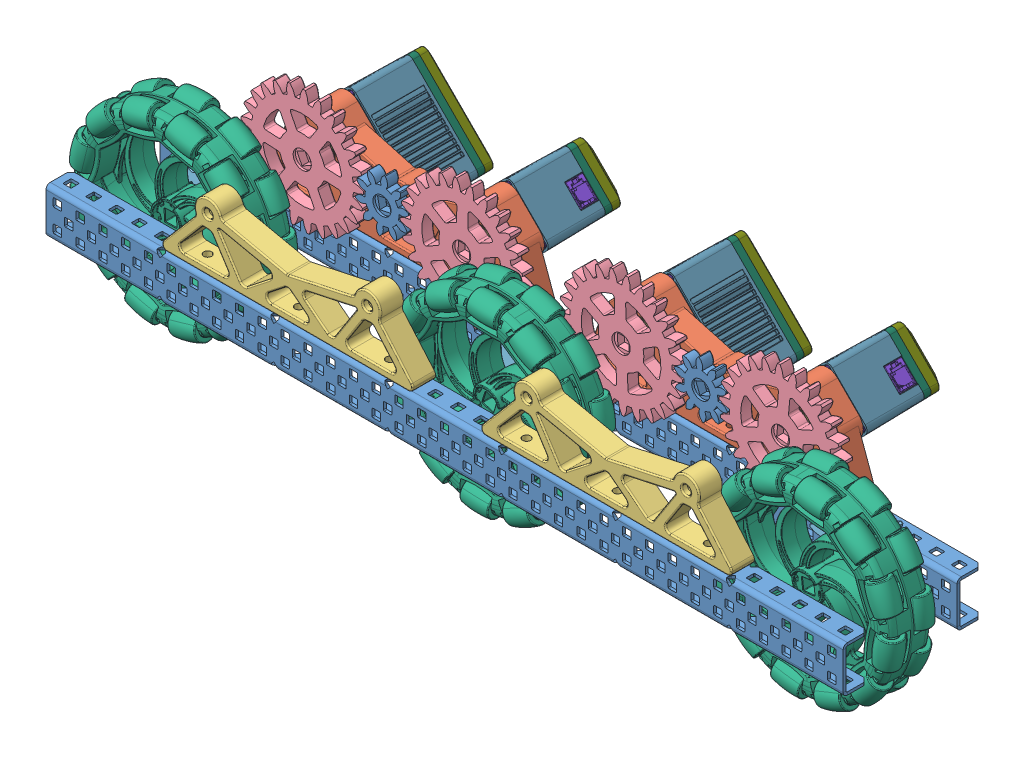
SolidWorks assembly Chassis_Side_assembly, configuration Default. Lengths in mm.
Overall size (477.85 153.68 124.38).
102 component instances, 19 part files, 62 mates.
Components (placement in the parent):
- 1x2x1x35 Aluminum C-Channel (276-2289)-1: 1x2x1x35 Aluminum C-Channel (276-2289) [Default] at (127.7015 217.7804 370.9956) size (444.5 25.41 13.97)
- 1x2x1x35 Aluminum C-Channel (276-2289)-2: 1x2x1x35 Aluminum C-Channel (276-2289) [Default] at (127.7015 217.7804 307.4956) size (444.5 25.41 13.97)
- chassis_inner_bracket-1: chassis_inner_bracket [Default] at (127.7015 224.1304 306.2256) x (-1 0 0) z (0 0 -1) size (150.69 49.95 15.04)
- chassis_inner_bracket-2: chassis_inner_bracket [Default] at (305.5015 224.1304 306.2256) x (-1 0 0) z (0 0 -1) size (150.69 49.95 15.04)
- chassis_outer_bracket-1: chassis_outer_bracket [Default] at (127.7015 224.1304 369.7256) x (-1 0 0) z (0 0 -1) size (139.7 37.07 12.7)
- chassis_outer_bracket-2: chassis_outer_bracket [Default] at (305.5015 224.1304 369.7256) x (-1 0 0) z (0 0 -1) size (139.7 37.07 12.7)
- ORION 10Pd 25T Gear-1: ORION 10Pd 25T Gear [Inch - Spur gear 10DP 25T 20PA 0.25FW ---S25N3.0H2.0L0.25N] at (-5.6485 260.0514 310.6706) x (0 0 1) z (0.890535 0.454914 0) size (6.39 68.44 68.58)
- ORION 10Pd 25T Gear-2: ORION 10Pd 25T Gear [Inch - Spur gear 10DP 25T 20PA 0.25FW ---S25N3.0H2.0L0.25N] at (83.2515 260.0514 310.6706) x (0 0 1) z (-0.999708 0.024179 0) size (6.39 68.44 68.58)
- ORION 10Pd 25T Gear-3: ORION 10Pd 25T Gear [Inch - Spur gear 10DP 25T 20PA 0.25FW ---S25N3.0H2.0L0.25N] at (172.1515 260.0514 310.6706) x (0 0 1) z (-0.999528 -0.030725 0) size (6.39 68.44 68.58)
- ORION 10Pd 25T Gear-4: ORION 10Pd 25T Gear [Inch - Spur gear 10DP 25T 20PA 0.25FW ---S25N3.0H2.0L0.25N] at (261.0515 260.0514 310.6706) x (0 0 1) z (-0.995159 0.098276 0) size (6.39 68.44 68.58)
- ORION 10Pd 20T Gear-1: ORION 10Pd 20T Gear [Inch - Spur gear 10DP 20T 20PA 0.25FW ---S20N3.0H2.0L0.25N] at (-50.0985 224.1304 310.6706) x (0 0 1) z (-0.999757 -0.022029 0) size (6.39 55.44 55.44)
- ORION 10Pd 20T Gear-2: ORION 10Pd 20T Gear [Inch - Spur gear 10DP 20T 20PA 0.25FW ---S20N3.0H2.0L0.25N] at (305.5015 224.1304 310.6706) x (0 0 1) z (0.992506 0.122196 0) size (6.39 55.44 55.44)
- ORION 10Pd 20T Gear-3: ORION 10Pd 20T Gear [Inch - Spur gear 10DP 20T 20PA 0.25FW ---S20N3.0H2.0L0.25N] at (127.7015 224.1304 310.6706) x (0 0 1) z (0.955092 -0.29631 0) size (6.39 55.44 55.44)
- 4_ Omni-Directional Wheel (276-2185) -1: 4_ Omni-Directional Wheel (276-2185)  [Default] at (-50.0985 224.1304 339.0206) x (0.022029 -0.999757 0) z (0.999757 0.022029 0) size (114.44 40.55 114.44)
- 4_ Omni-Directional Wheel (276-2185) -2: 4_ Omni-Directional Wheel (276-2185)  [Default] at (127.7015 224.1304 339.0206) x (-0.955092 0.29631 0) z (-0.29631 -0.955092 0) size (114.44 40.55 114.44)
- 4_ Omni-Directional Wheel (276-2185) -3: 4_ Omni-Directional Wheel (276-2185)  [Default] at (305.5015 224.1304 339.0206) x (-0.992506 -0.122196 0) z (0.122196 -0.992506 0) size (114.44 40.55 114.44)
- V5 Smart Motor (276-4840) no cap-1: V5 Smart Motor (276-4840) no cap [Default] at (252.0713 251.0711 274.0256) x (0.707107 0.707107 0) z (0 0 1) size (59.01 35.33 59.91)
  - V5 Smart Motor (276-4840).step-1: V5 Smart Motor (276-4840).step [Default] at origin size (59.01 35.33 59.91)
    - 276-4840-900 Rev6_Instruction.step-1: 276-4840-900 Rev6_Instruction.step [Default] at (-14.3 0 -17.2) size (52.79 15.94 38.15)
      - 276-4840-901 Rev6.step-1: 276-4840-901 Rev6.step [Default] at (10.75 -10.05 17.8) x (-1 0 0) z (0 0 1) size (49.9 1.6 38.15)
      - 276-4840-902 Rev2.step-1: 276-4840-902 Rev2.step [Default] at (31.25 -9.25 6.2) x (0 0 -1) z (0 -1 0) size (10.35 11.39 15.94)
      - 276-4840-022 Rev4.step-1: 276-4840-022 Rev4.step [Default] at (31.25 -9.25 6.2) x (0 0 -1) z (1 0 0) size (10.26 9.1 5.51)
    - 276-4840-110 Rev10_Instruction.step-1: 276-4840-110 Rev10_Instruction.step [Default] at (12.7 0 14.7) size (35.33 35.33 31.1)
      - 276-4840-061 Rev7_Ring_Gear_Fixed01 .6 Rev3.step-1: 276-4840-061 Rev7_Ring_Gear_Fixed01 .6 Rev3.step [Default] at origin size (28.79 28.39 24.6)
      - 276-4840-018 Rev6.step-1: 276-4840-018 Rev6.step [Default] at (0 0 6.7) x (-0.483174 0.875524 0) z (0 0 1) size (26 26 12.3)
      - 276-4840-059 Rev2.step-1: 276-4840-059 Rev2.step [Default] at (0 0 10.3) size (28.4 28.4 8.5)
      - 276-4840-062 Rev1.step-1: 276-4840-062 Rev1.step [Default] at (-12.1353 8.8168 12.3) x (0.956835 -0.290632 0) z (-0.290632 -0.956835 0) size (3.2 6.56 3.2)
      - 276-4840-062 Rev1.step-2: 276-4840-062 Rev1.step [Default] at (12.1353 8.8168 12.3) x (0.978427 0.206591 0) z (0.206591 -0.978427 0) size (3.2 6.56 3.2)
      - 276-4840-062 Rev1.step-3: 276-4840-062 Rev1.step [Default] at (-12.1353 -8.8168 12.3) x (0.72563 0.688086 0) z (0.688086 -0.72563 0) size (3.2 6.56 3.2)
    - 276-4840-001 Rev38.step-1: 276-4840-001 Rev38.step [Default] at origin size (57.3 33 46.9)
    - 276-4840-005 Rev27.step-1: 276-4840-005 Rev27.step [Default] at (0 0 -17.95) size (56.17 31.87 12.9)
    - 276-4840-004 Rev16.step-1: 276-4840-004 Rev16.step [Default] at (0 0 -19.2) size (56.01 31.71 9.21)
    - 276-4840-009 Rev3.step-1: 276-4840-009 Rev3.step [Default] at (25.45 13.5 15.7) x (0.19987 -0.979823 0) z (-0.979823 -0.19987 0) size (3.4 41.31 4.34)
    - 276-4840-009 Rev3.step-2: 276-4840-009 Rev3.step [Default] at (-25.45 -13.5 15.7) x (-0.998855 0.047836 0) z (0.047836 0.998855 0) size (3.4 41.31 4.34)
    - 276-4840-009 Rev3.step-3: 276-4840-009 Rev3.step [Default] at (25.45 -13.5 15.7) x (-0.975374 0.220559 0) z (0.220559 0.975374 0) size (3.4 41.31 4.34)
    - 276-4840-009 Rev3.step-4: 276-4840-009 Rev3.step [Default] at (-25.45 13.5 15.7) x (-0.922256 0.38658 0) z (0.38658 0.922256 0) size (3.4 41.31 4.34)
    - 276-4840-025 Rev19.step-1: 276-4840-025 Rev19.step [Default] at (12.7 0 -22.63) x (-0.993315 0.115437 0) z (0 0 1) size (14.82 14.83 35.18)
- V5 Smart Motor (276-4840) no cap-2: V5 Smart Motor (276-4840) no cap [Default] at (181.1318 251.0711 274.0256) x (-0.707107 0.707107 0) z (0 0 1) size (59.01 35.33 59.91)
  - V5 Smart Motor (276-4840).step-1: V5 Smart Motor (276-4840).step [Default] at origin size (59.01 35.33 59.91)
    - 276-4840-900 Rev6_Instruction.step-1: 276-4840-900 Rev6_Instruction.step [Default] at (-14.3 0 -17.2) size (52.79 15.94 38.15)
      - 276-4840-901 Rev6.step-1: 276-4840-901 Rev6.step [Default] at (10.75 -10.05 17.8) x (-1 0 0) z (0 0 1) size (49.9 1.6 38.15)
      - 276-4840-902 Rev2.step-1: 276-4840-902 Rev2.step [Default] at (31.25 -9.25 6.2) x (0 0 -1) z (0 -1 0) size (10.35 11.39 15.94)
      - 276-4840-022 Rev4.step-1: 276-4840-022 Rev4.step [Default] at (31.25 -9.25 6.2) x (0 0 -1) z (1 0 0) size (10.26 9.1 5.51)
    - 276-4840-110 Rev10_Instruction.step-1: 276-4840-110 Rev10_Instruction.step [Default] at (12.7 0 14.7) size (35.33 35.33 31.1)
      - 276-4840-061 Rev7_Ring_Gear_Fixed01 .6 Rev3.step-1: 276-4840-061 Rev7_Ring_Gear_Fixed01 .6 Rev3.step [Default] at origin size (28.79 28.39 24.6)
      - 276-4840-018 Rev6.step-1: 276-4840-018 Rev6.step [Default] at (0 0 6.7) x (-0.483174 0.875524 0) z (0 0 1) size (26 26 12.3)
      - 276-4840-059 Rev2.step-1: 276-4840-059 Rev2.step [Default] at (0 0 10.3) size (28.4 28.4 8.5)
      - 276-4840-062 Rev1.step-1: 276-4840-062 Rev1.step [Default] at (-12.1353 8.8168 12.3) x (0.956835 -0.290632 0) z (-0.290632 -0.956835 0) size (3.2 6.56 3.2)
      - 276-4840-062 Rev1.step-2: 276-4840-062 Rev1.step [Default] at (12.1353 8.8168 12.3) x (0.978427 0.206591 0) z (0.206591 -0.978427 0) size (3.2 6.56 3.2)
      - 276-4840-062 Rev1.step-3: 276-4840-062 Rev1.step [Default] at (-12.1353 -8.8168 12.3) x (0.72563 0.688086 0) z (0.688086 -0.72563 0) size (3.2 6.56 3.2)
    - 276-4840-001 Rev38.step-1: 276-4840-001 Rev38.step [Default] at origin size (57.3 33 46.9)
    - 276-4840-005 Rev27.step-1: 276-4840-005 Rev27.step [Default] at (0 0 -17.95) size (56.17 31.87 12.9)
    - 276-4840-004 Rev16.step-1: 276-4840-004 Rev16.step [Default] at (0 0 -19.2) size (56.01 31.71 9.21)
    - 276-4840-009 Rev3.step-1: 276-4840-009 Rev3.step [Default] at (25.45 13.5 15.7) x (0.19987 -0.979823 0) z (-0.979823 -0.19987 0) size (3.4 41.31 4.34)
    - 276-4840-009 Rev3.step-2: 276-4840-009 Rev3.step [Default] at (-25.45 -13.5 15.7) x (-0.998855 0.047836 0) z (0.047836 0.998855 0) size (3.4 41.31 4.34)
    - 276-4840-009 Rev3.step-3: 276-4840-009 Rev3.step [Default] at (25.45 -13.5 15.7) x (-0.975374 0.220559 0) z (0.220559 0.975374 0) size (3.4 41.31 4.34)
    - 276-4840-009 Rev3.step-4: 276-4840-009 Rev3.step [Default] at (-25.45 13.5 15.7) x (-0.922256 0.38658 0) z (0.38658 0.922256 0) size (3.4 41.31 4.34)
    - 276-4840-025 Rev19.step-1: 276-4840-025 Rev19.step [Default] at (12.7 0 -22.63) x (-0.993315 0.115437 0) z (0 0 1) size (14.82 14.83 35.18)
- V5 Smart Motor (276-4840) no cap-3: V5 Smart Motor (276-4840) no cap [Default] at (74.2713 251.0711 274.0256) x (0.707107 0.707107 0) z (0 0 1) size (59.01 35.33 59.91)
  - V5 Smart Motor (276-4840).step-1: V5 Smart Motor (276-4840).step [Default] at origin size (59.01 35.33 59.91)
    - 276-4840-900 Rev6_Instruction.step-1: 276-4840-900 Rev6_Instruction.step [Default] at (-14.3 0 -17.2) size (52.79 15.94 38.15)
      - 276-4840-901 Rev6.step-1: 276-4840-901 Rev6.step [Default] at (10.75 -10.05 17.8) x (-1 0 0) z (0 0 1) size (49.9 1.6 38.15)
      - 276-4840-902 Rev2.step-1: 276-4840-902 Rev2.step [Default] at (31.25 -9.25 6.2) x (0 0 -1) z (0 -1 0) size (10.35 11.39 15.94)
      - 276-4840-022 Rev4.step-1: 276-4840-022 Rev4.step [Default] at (31.25 -9.25 6.2) x (0 0 -1) z (1 0 0) size (10.26 9.1 5.51)
    - 276-4840-110 Rev10_Instruction.step-1: 276-4840-110 Rev10_Instruction.step [Default] at (12.7 0 14.7) size (35.33 35.33 31.1)
      - 276-4840-061 Rev7_Ring_Gear_Fixed01 .6 Rev3.step-1: 276-4840-061 Rev7_Ring_Gear_Fixed01 .6 Rev3.step [Default] at origin size (28.79 28.39 24.6)
      - 276-4840-018 Rev6.step-1: 276-4840-018 Rev6.step [Default] at (0 0 6.7) x (-0.483174 0.875524 0) z (0 0 1) size (26 26 12.3)
      - 276-4840-059 Rev2.step-1: 276-4840-059 Rev2.step [Default] at (0 0 10.3) size (28.4 28.4 8.5)
      - 276-4840-062 Rev1.step-1: 276-4840-062 Rev1.step [Default] at (-12.1353 8.8168 12.3) x (0.956835 -0.290632 0) z (-0.290632 -0.956835 0) size (3.2 6.56 3.2)
      - 276-4840-062 Rev1.step-2: 276-4840-062 Rev1.step [Default] at (12.1353 8.8168 12.3) x (0.978427 0.206591 0) z (0.206591 -0.978427 0) size (3.2 6.56 3.2)
      - 276-4840-062 Rev1.step-3: 276-4840-062 Rev1.step [Default] at (-12.1353 -8.8168 12.3) x (0.72563 0.688086 0) z (0.688086 -0.72563 0) size (3.2 6.56 3.2)
    - 276-4840-001 Rev38.step-1: 276-4840-001 Rev38.step [Default] at origin size (57.3 33 46.9)
    - 276-4840-005 Rev27.step-1: 276-4840-005 Rev27.step [Default] at (0 0 -17.95) size (56.17 31.87 12.9)
    - 276-4840-004 Rev16.step-1: 276-4840-004 Rev16.step [Default] at (0 0 -19.2) size (56.01 31.71 9.21)
    - 276-4840-009 Rev3.step-1: 276-4840-009 Rev3.step [Default] at (25.45 13.5 15.7) x (0.19987 -0.979823 0) z (-0.979823 -0.19987 0) size (3.4 41.31 4.34)
    - 276-4840-009 Rev3.step-2: 276-4840-009 Rev3.step [Default] at (-25.45 -13.5 15.7) x (-0.998855 0.047836 0) z (0.047836 0.998855 0) size (3.4 41.31 4.34)
    - 276-4840-009 Rev3.step-3: 276-4840-009 Rev3.step [Default] at (25.45 -13.5 15.7) x (-0.975374 0.220559 0) z (0.220559 0.975374 0) size (3.4 41.31 4.34)
    - 276-4840-009 Rev3.step-4: 276-4840-009 Rev3.step [Default] at (-25.45 13.5 15.7) x (-0.922256 0.38658 0) z (0.38658 0.922256 0) size (3.4 41.31 4.34)
    - 276-4840-025 Rev19.step-1: 276-4840-025 Rev19.step [Default] at (12.7 0 -22.63) x (-0.993315 0.115437 0) z (0 0 1) size (14.82 14.83 35.18)
- V5 Smart Motor (276-4840) no cap-4: V5 Smart Motor (276-4840) no cap [Default] at (3.3318 251.0711 274.0256) x (-0.707107 0.707107 0) z (0 0 1) size (59.01 35.33 59.91)
  - V5 Smart Motor (276-4840).step-1: V5 Smart Motor (276-4840).step [Default] at origin size (59.01 35.33 59.91)
    - 276-4840-900 Rev6_Instruction.step-1: 276-4840-900 Rev6_Instruction.step [Default] at (-14.3 0 -17.2) size (52.79 15.94 38.15)
      - 276-4840-901 Rev6.step-1: 276-4840-901 Rev6.step [Default] at (10.75 -10.05 17.8) x (-1 0 0) z (0 0 1) size (49.9 1.6 38.15)
      - 276-4840-902 Rev2.step-1: 276-4840-902 Rev2.step [Default] at (31.25 -9.25 6.2) x (0 0 -1) z (0 -1 0) size (10.35 11.39 15.94)
      - 276-4840-022 Rev4.step-1: 276-4840-022 Rev4.step [Default] at (31.25 -9.25 6.2) x (0 0 -1) z (1 0 0) size (10.26 9.1 5.51)
    - 276-4840-110 Rev10_Instruction.step-1: 276-4840-110 Rev10_Instruction.step [Default] at (12.7 0 14.7) size (35.33 35.33 31.1)
      - 276-4840-061 Rev7_Ring_Gear_Fixed01 .6 Rev3.step-1: 276-4840-061 Rev7_Ring_Gear_Fixed01 .6 Rev3.step [Default] at origin size (28.79 28.39 24.6)
      - 276-4840-018 Rev6.step-1: 276-4840-018 Rev6.step [Default] at (0 0 6.7) x (-0.483174 0.875524 0) z (0 0 1) size (26 26 12.3)
      - 276-4840-059 Rev2.step-1: 276-4840-059 Rev2.step [Default] at (0 0 10.3) size (28.4 28.4 8.5)
      - 276-4840-062 Rev1.step-1: 276-4840-062 Rev1.step [Default] at (-12.1353 8.8168 12.3) x (0.956835 -0.290632 0) z (-0.290632 -0.956835 0) size (3.2 6.56 3.2)
      - 276-4840-062 Rev1.step-2: 276-4840-062 Rev1.step [Default] at (12.1353 8.8168 12.3) x (0.978427 0.206591 0) z (0.206591 -0.978427 0) size (3.2 6.56 3.2)
      - 276-4840-062 Rev1.step-3: 276-4840-062 Rev1.step [Default] at (-12.1353 -8.8168 12.3) x (0.72563 0.688086 0) z (0.688086 -0.72563 0) size (3.2 6.56 3.2)
    - 276-4840-001 Rev38.step-1: 276-4840-001 Rev38.step [Default] at origin size (57.3 33 46.9)
    - 276-4840-005 Rev27.step-1: 276-4840-005 Rev27.step [Default] at (0 0 -17.95) size (56.17 31.87 12.9)
    - 276-4840-004 Rev16.step-1: 276-4840-004 Rev16.step [Default] at (0 0 -19.2) size (56.01 31.71 9.21)
    - 276-4840-009 Rev3.step-1: 276-4840-009 Rev3.step [Default] at (25.45 13.5 15.7) x (0.19987 -0.979823 0) z (-0.979823 -0.19987 0) size (3.4 41.31 4.34)
    - 276-4840-009 Rev3.step-2: 276-4840-009 Rev3.step [Default] at (-25.45 -13.5 15.7) x (-0.998855 0.047836 0) z (0.047836 0.998855 0) size (3.4 41.31 4.34)
    - 276-4840-009 Rev3.step-3: 276-4840-009 Rev3.step [Default] at (25.45 -13.5 15.7) x (-0.975374 0.220559 0) z (0.220559 0.975374 0) size (3.4 41.31 4.34)
    - 276-4840-009 Rev3.step-4: 276-4840-009 Rev3.step [Default] at (-25.45 13.5 15.7) x (-0.922256 0.38658 0) z (0.38658 0.922256 0) size (3.4 41.31 4.34)
    - 276-4840-025 Rev19.step-1: 276-4840-025 Rev19.step [Default] at (12.7 0 -22.63) x (-0.993315 0.115437 0) z (0 0 1) size (14.82 14.83 35.18)
- ORION 10Pd 10T Gear-3: ORION 10Pd 10T Gear [Inch - Spur gear 10DP 10T 20PA 0.25inFW ---S10N3.0H2.0L0.25N] at (38.8015 260.0514 310.6706) x (0 0 1) z (-0.977332 -0.211714 0) size (6.4 29.22 30.53)
- ORION 10Pd 10T Gear-4: ORION 10Pd 10T Gear [Inch - Spur gear 10DP 10T 20PA 0.25inFW ---S10N3.0H2.0L0.25N] at (216.6015 260.0514 310.6706) x (0 0 1) z (-0.923728 -0.383049 0) size (6.4 29.22 30.53)
Mates (geometry in assembly coordinates):
- Coincident1: coincident anti-aligned: plane of 1x2x1x35 Aluminum C-Channel (276-2289)-1 through (-94.0485 230.4804 403.3543) normal (0 1 0); plane of chassis_outer_bracket-1 through (127.7015 230.4804 357.0256) normal (0 -1 0)
- Coincident2: coincident aligned: plane of 1x2x1x35 Aluminum C-Channel (276-2289)-1 through (-92.0604 228.9056 357.0256) normal (0 0 -1); plane of chassis_outer_bracket-1 through (127.7015 224.1304 357.0256) normal (0 0 -1)
- Coincident3: coincident aligned: plane of 1x2x1x35 Aluminum C-Channel (276-2289)-1 through (161.9396 228.9056 357.0256) normal (0 0 -1); plane of chassis_outer_bracket-2 through (305.5015 224.1304 357.0256) normal (0 0 -1)
- Coincident4: coincident anti-aligned: plane of 1x2x1x35 Aluminum C-Channel (276-2289)-1 through (-94.0485 230.4804 403.3543) normal (0 1 0); plane of chassis_outer_bracket-2 through (305.5015 230.4804 357.0256) normal (0 -1 0)
- Concentric1: concentric anti-aligned: circle of 1x2x1x35 Aluminum C-Channel (276-2289)-1; cylinder of chassis_outer_bracket-1 through (-11.9985 267.5524 363.3756) axis (0 -1 0) radius 2.2
- Concentric2: concentric anti-aligned: circle of 1x2x1x35 Aluminum C-Channel (276-2289)-1; cylinder of chassis_outer_bracket-2 through (267.4015 267.5524 363.3756) axis (0 -1 0) radius 2.2
- Coincident5: coincident aligned: plane of 1x2x1x35 Aluminum C-Channel (276-2289)-1 through (-94.0485 230.4804 403.3543) normal (0 1 0); plane of 1x2x1x35 Aluminum C-Channel (276-2289)-2 through (-94.0485 230.4804 339.8543) normal (0 1 0)
- Coincident6: coincident: line of 1x2x1x35 Aluminum C-Channel (276-2289)-1 through (-94.5485 207.468 369.4208) axis (0 1 0); plane of 1x2x1x35 Aluminum C-Channel (276-2289)-2 through (-94.5485 195.8601 305.9208) normal (-1 0 0)
- Distance1: distance = 63.5 mm: point of 1x2x1x35 Aluminum C-Channel (276-2289)-2; point of 1x2x1x35 Aluminum C-Channel (276-2289)-1
- Coincident8: coincident anti-aligned: plane of 1x2x1x35 Aluminum C-Channel (276-2289)-2 through (-94.0485 230.4804 339.8543) normal (0 1 0); plane of chassis_inner_bracket-1 through (127.7015 230.4804 293.5256) normal (0 -1 0)
- Coincident9: coincident anti-aligned: plane of 1x2x1x35 Aluminum C-Channel (276-2289)-2 through (-94.0485 230.4804 339.8543) normal (0 1 0); plane of chassis_inner_bracket-2 through (305.5015 230.4804 293.5256) normal (0 -1 0)
- Concentric3: concentric aligned: circle of chassis_inner_bracket-2; circle of chassis_outer_bracket-2
- Concentric4: concentric anti-aligned: circle of 1x2x1x35 Aluminum C-Channel (276-2289)-2; cylinder of chassis_inner_bracket-2 through (267.4015 280.4268 299.8756) axis (0 -1 0) radius 2.2
- Concentric5: concentric aligned: circle of chassis_inner_bracket-1; circle of chassis_outer_bracket-1
- Concentric6: concentric anti-aligned: circle of 1x2x1x35 Aluminum C-Channel (276-2289)-2; circle of chassis_inner_bracket-1
- Concentric7: concentric anti-aligned: circle of chassis_inner_bracket-1; circle of ORION 10Pd 25T Gear-1
- Concentric8: concentric anti-aligned: circle of chassis_inner_bracket-1; circle of ORION 10Pd 25T Gear-2
- Concentric11: concentric anti-aligned: circle of chassis_inner_bracket-2; circle of ORION 10Pd 25T Gear-3
- Concentric12: concentric anti-aligned: circle of chassis_inner_bracket-2; circle of ORION 10Pd 25T Gear-4
- Concentric13: concentric aligned: circle of 1x2x1x35 Aluminum C-Channel (276-2289)-2; circle of ORION 10Pd 20T Gear-1
- Coincident14: coincident aligned: plane of ORION 10Pd 25T Gear-1 through (-5.6485 260.0514 317.0206) normal (0 0 1); plane of ORION 10Pd 20T Gear-1 through (-50.0985 224.1304 317.0206) normal (0 0 1)
- Coincident15: coincident aligned: plane of ORION 10Pd 25T Gear-4 through (261.0515 260.0514 310.6706) normal (0 0 -1); plane of ORION 10Pd 20T Gear-2 through (305.5015 224.1304 310.6706) normal (0 0 -1)
- Concentric14: concentric aligned: circle of 1x2x1x35 Aluminum C-Channel (276-2289)-2; circle of ORION 10Pd 20T Gear-2
- Coincident16: coincident aligned: plane of ORION 10Pd 25T Gear-2 through (83.2515 260.0514 317.0206) normal (0 0 1); plane of ORION 10Pd 25T Gear-3 through (172.1515 260.0514 317.0206) normal (0 0 1)
- Coincident17: coincident aligned: plane of ORION 10Pd 25T Gear-2 through (83.2515 260.0514 310.6706) normal (0 0 -1); plane of ORION 10Pd 20T Gear-3 through (127.7015 224.1304 310.6706) normal (0 0 -1)
- Concentric15: concentric aligned: circle of 1x2x1x35 Aluminum C-Channel (276-2289)-2; circle of ORION 10Pd 20T Gear-3
- GearMate2: gear = 57.1475 : 44.4475 mm: circle of ORION 10Pd 20T Gear-1; circle of ORION 10Pd 25T Gear-1
- GearMate5: gear = 44.4475 : 57.1475 mm: circle of ORION 10Pd 25T Gear-2; circle of ORION 10Pd 20T Gear-3
- GearMate6: gear = 44.4475 : 57.1475 mm: circle of ORION 10Pd 25T Gear-3; circle of ORION 10Pd 20T Gear-3
- GearMate9: gear = 44.4475 : 57.1475 mm: circle of ORION 10Pd 25T Gear-4; circle of ORION 10Pd 20T Gear-2
- Distance2: distance = 3.175 mm anti-aligned: plane of ORION 10Pd 20T Gear-1 through (-50.0985 224.1304 310.6706) normal (0 0 -1); plane of 1x2x1x35 Aluminum C-Channel (276-2289)-2 through (-94.0485 195.8601 307.4956) normal (0 0 1)
- Concentric18: concentric anti-aligned: circle of ORION 10Pd 20T Gear-1; circle of 4_ Omni-Directional Wheel (276-2185) -1
- Coincident19: coincident aligned: plane of ORION 10Pd 20T Gear-1 through (-53.2727 224.0604 311.9406) normal (0.999757 0.022029 0); plane of 4_ Omni-Directional Wheel (276-2185) -1 through (-53.2027 220.8862 352.0242) normal (0.999757 0.022029 0)
- Concentric19: concentric anti-aligned: circle of ORION 10Pd 20T Gear-3; circle of 4_ Omni-Directional Wheel (276-2185) -2
- Coincident20: coincident aligned: plane of ORION 10Pd 20T Gear-3 through (128.6423 227.1628 311.9406) normal (-0.29631 -0.955092 0); plane of 4_ Omni-Directional Wheel (276-2185) -2 through (125.6099 228.1036 352.0242) normal (-0.29631 -0.955092 0)
- Concentric20: concentric anti-aligned: circle of ORION 10Pd 20T Gear-2; circle of 4_ Omni-Directional Wheel (276-2185) -3
- Coincident21: coincident aligned: plane of ORION 10Pd 20T Gear-2 through (305.1136 227.2816 311.9406) normal (0.122196 -0.992506 0); plane of 4_ Omni-Directional Wheel (276-2185) -3 through (301.9624 226.8936 352.0242) normal (0.122196 -0.992506 0)
- Distance3: distance = 15 mm anti-aligned: plane of 4_ Omni-Directional Wheel (276-2185) -1 through (-50.0985 224.1304 332.0206) normal (0 0 -1); plane of ORION 10Pd 20T Gear-1 through (-50.0985 224.1304 317.0206) normal (0 0 1)
- Coincident23: coincident aligned: plane of 4_ Omni-Directional Wheel (276-2185) -1 through (-50.0985 224.1304 346.0206) normal (0 0 1); plane of 4_ Omni-Directional Wheel (276-2185) -2 through (127.7015 224.1304 346.0206) normal (0 0 1)
- Coincident24: coincident aligned: plane of 4_ Omni-Directional Wheel (276-2185) -2 through (127.7015 224.1304 346.0206) normal (0 0 1); plane of 4_ Omni-Directional Wheel (276-2185) -3 through (305.5015 224.1304 346.0206) normal (0 0 1)
- Concentric21: concentric aligned: cylinder of chassis_inner_bracket-2 through (243.091 242.0909 293.5256) axis (0 0 1) radius 4.3; circle of V5 Smart Motor (276-4840) no cap-1/V5 Smart Motor (276-4840).step-1/276-4840-001 Rev38.step-1
- Parallel1: parallel anti-aligned: line of chassis_inner_bracket-2 through (267.062 278.0826 291.2256) axis (0.707107 -0.707107 0); line of V5 Smart Motor (276-4840) no cap-1/V5 Smart Motor (276-4840).step-1/276-4840-001 Rev38.step-1 through (281.4516 262.2081 290.2256) axis (-0.707107 0.707107 0)
- Coincident26: coincident anti-aligned: plane of chassis_inner_bracket-2 through (305.5015 224.1304 291.2256) normal (0 0 -1); plane of V5 Smart Motor (276-4840) no cap-1/V5 Smart Motor (276-4840).step-1/276-4840-001 Rev38.step-1 through (225.2366 242.4798 291.2256) normal (0 0 1)
- Concentric22: concentric anti-aligned: circle of chassis_inner_bracket-2; circle of V5 Smart Motor (276-4840) no cap-2/V5 Smart Motor (276-4840).step-1/276-4840-001 Rev38.step-1
- Parallel2: parallel anti-aligned: line of chassis_inner_bracket-2 through (155.5345 264.6476 291.2256) axis (0.707107 0.707107 0); line of V5 Smart Motor (276-4840) no cap-2/V5 Smart Motor (276-4840).step-1/276-4840-001 Rev38.step-1 through (169.9949 280.4514 290.2256) axis (-0.707107 -0.707107 0)
- Coincident28: coincident anti-aligned: plane of chassis_inner_bracket-2 through (305.5015 224.1304 291.2256) normal (0 0 -1); plane of V5 Smart Motor (276-4840) no cap-2/V5 Smart Motor (276-4840).step-1/276-4840-001 Rev38.step-1 through (189.7231 224.2364 291.2256) normal (0 0 1)
- Concentric23: concentric aligned: circle of chassis_inner_bracket-1; circle of V5 Smart Motor (276-4840) no cap-3/V5 Smart Motor (276-4840).step-1/276-4840-001 Rev38.step-1
- Parallel3: parallel anti-aligned: line of chassis_inner_bracket-1 through (89.262 278.0826 291.2256) axis (0.707107 -0.707107 0); line of V5 Smart Motor (276-4840) no cap-3/V5 Smart Motor (276-4840).step-1/276-4840-001 Rev38.step-1 through (103.6516 262.2081 290.2256) axis (-0.707107 0.707107 0)
- Coincident30: coincident anti-aligned: plane of chassis_inner_bracket-1 through (127.7015 224.1304 291.2256) normal (0 0 -1); plane of V5 Smart Motor (276-4840) no cap-3/V5 Smart Motor (276-4840).step-1/276-4840-001 Rev38.step-1 through (47.4366 242.4798 291.2256) normal (0 0 1)
- Concentric24: concentric aligned: circle of chassis_inner_bracket-1; circle of V5 Smart Motor (276-4840) no cap-4/V5 Smart Motor (276-4840).step-1/276-4840-001 Rev38.step-1
- Parallel4: parallel anti-aligned: line of chassis_inner_bracket-1 through (-22.2655 264.6476 291.2256) axis (0.707107 0.707107 0); line of V5 Smart Motor (276-4840) no cap-4/V5 Smart Motor (276-4840).step-1/276-4840-001 Rev38.step-1 through (-7.8051 280.4514 290.2256) axis (-0.707107 -0.707107 0)
- Coincident32: coincident anti-aligned: plane of chassis_inner_bracket-1 through (127.7015 224.1304 291.2256) normal (0 0 -1); plane of V5 Smart Motor (276-4840) no cap-4/V5 Smart Motor (276-4840).step-1/276-4840-001 Rev38.step-1 through (11.9231 224.2364 291.2256) normal (0 0 1)
- Coincident33: coincident aligned: plane of ORION 10Pd 25T Gear-2 through (83.2515 260.0514 310.6706) normal (0 0 -1); plane of ORION 10Pd 10T Gear-3 through (38.8015 260.0514 310.6706) normal (0 0 -1)
- Coincident34: coincident aligned: plane of ORION 10Pd 25T Gear-4 through (261.0515 260.0514 310.6706) normal (0 0 -1); plane of ORION 10Pd 10T Gear-4 through (216.6015 260.0514 310.6706) normal (0 0 -1)
- Concentric25: concentric anti-aligned: circle of chassis_inner_bracket-1; circle of ORION 10Pd 10T Gear-3
- Coincident35: coincident aligned: plane of ORION 10Pd 25T Gear-1 through (-5.6485 260.0514 317.0206) normal (0 0 1); plane of ORION 10Pd 10T Gear-3 through (38.8015 260.0514 317.0206) normal (0 0 1)
- Concentric26: concentric anti-aligned: circle of chassis_inner_bracket-2; circle of ORION 10Pd 10T Gear-4
- GearMate10: gear = 57.1475 : 19.0475 mm: circle of ORION 10Pd 10T Gear-3; circle of ORION 10Pd 25T Gear-2
- GearMate11: gear = 57.1475 : 19.0475 mm: circle of ORION 10Pd 10T Gear-3; circle of ORION 10Pd 25T Gear-1
- GearMate12: gear = 57.1475 : 19.0475 mm: circle of ORION 10Pd 10T Gear-4; circle of ORION 10Pd 25T Gear-3
- Coincident36: coincident aligned: plane of ORION 10Pd 25T Gear-3 through (172.1515 260.0514 317.0206) normal (0 0 1); plane of ORION 10Pd 10T Gear-4 through (216.6015 260.0514 317.0206) normal (0 0 1)
- GearMate14: gear = 19.0475 : 57.1475 mm: circle of ORION 10Pd 25T Gear-4; circle of ORION 10Pd 10T Gear-4
